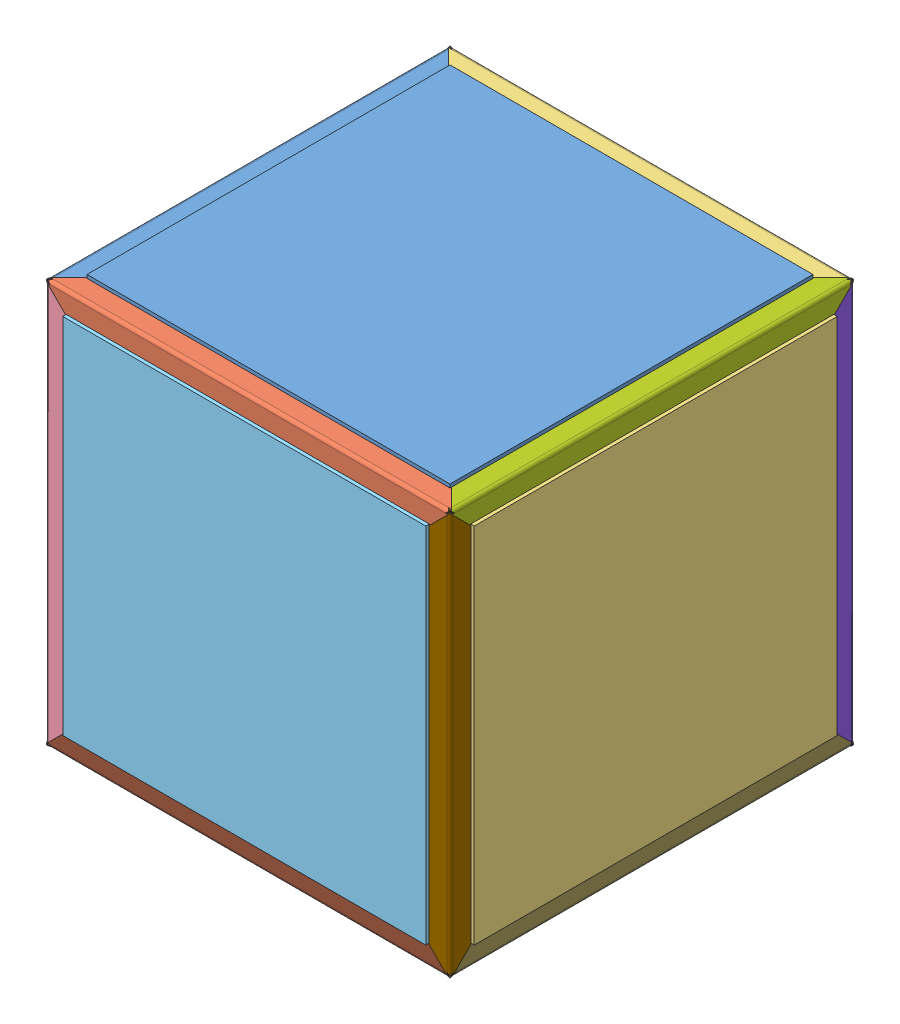
SolidWorks assembly cube_36, configuration cube36. Lengths in mm.
Overall size (188.59 188.59 188.59).
30 component instances, 30 part files, 93 mates.
Components (placement in the parent):
- pr^cube_36-28: pr^cube_36 [cube01] x (-1 0 0) z (0 0 1) size (166.37 1.59 166.37) (virtual)
- pg^cube_36-20: pg^cube_36 [cube01] x (0 -1 0) z (0 0 1) size (166.37 1.59 166.37) (virtual)
- po^cube_36-22: po^cube_36 [cube01] x (0 1 0) z (0 0 1) size (166.37 1.59 166.37) (virtual)
- py^cube_36-21: py^cube_36 [cube01] at origin size (166.37 1.59 166.37) (virtual)
- pc^cube_36-18: pc^cube_36 [cube01] x (-1 0 0) z (0 -1 0) size (166.37 1.59 166.37) (virtual)
- pb^cube_36-21: pb^cube_36 [cube01] x (-1 0 0) z (0 1 0) size (166.37 1.59 166.37) (virtual)
- br1^cube_36-49: br1^cube_36 [Default] at (0 67.31 -67.31) x (0 0 1) z (-1 0 0) size (50.8 50.8 127.51) (virtual)
- br2^cube_36-61: br2^cube_36 [Default] at (-67.31 67.31 0) size (50.8 50.8 127.51) (virtual)
- br3^cube_36-46: br3^cube_36 [Default] at (0 67.31 67.31) x (0 0 -1) z (1 0 0) size (50.8 50.8 127.51) (virtual)
- bg1^cube_36-47: bg1^cube_36 [Default] at (-67.31 -67.31 0) x (0 1 0) z (0 0 1) size (50.8 50.8 127.51) (virtual)
- bg2^cube_36-44: bg2^cube_36 [Default] at (-67.31 0 67.31) x (0 0 -1) z (0 1 0) size (50.8 50.8 127.51) (virtual)
- bg3^cube_36-40: bg3^cube_36 [Default] at (-67.31 0 -67.31) x (0 0 1) z (0 -1 0) size (50.8 50.8 127.51) (virtual)
- bo1^cube_36-42: bo1^cube_36 [Default] at (67.31 0 -67.31) x (0 0 1) z (0 1 0) size (50.8 50.8 127.51) (virtual)
- bo2^cube_36-46: bo2^cube_36 [Default] at (67.31 0 67.31) x (0 0 -1) z (0 -1 0) size (50.8 50.8 127.51) (virtual)
- bo3^cube_36-62: bo3^cube_36 [Default] at (67.31 67.31 0) x (0 -1 0) z (0 0 1) size (50.8 50.8 127.51) (virtual)
- by1^cube_36-41: by1^cube_36 [Default] at (0 -67.31 -67.31) x (0 0 1) z (1 0 0) size (50.8 50.8 127.51) (virtual)
- by2^cube_36-45: by2^cube_36 [Default] at (0 -67.31 67.31) x (0 0 -1) z (-1 0 0) size (50.8 50.8 127.51) (virtual)
- by3^cube_36-48: by3^cube_36 [Default] at (67.31 -67.31 0) x (-1 0 0) z (0 0 1) size (50.8 50.8 127.51) (virtual)
- dr1^cube_36-55: dr1^cube_36 [cube01] at (-92.1046 92.71 0) x (0 -1 0) z (0 0 1) size (26.01 26.01 185.43) (hidden, virtual)
- dr2^cube_36-37: dr2^cube_36 [cube01] at (0 92.71 92.1046) x (0 -1 0) z (1 0 0) size (26.01 26.01 185.43) (hidden, virtual)
- dr3^cube_36-33: dr3^cube_36 [cube01] at (0 92.71 -92.1046) x (0 -1 0) z (-1 0 0) size (26.01 26.01 185.43) (hidden, virtual)
- dg1^cube_36-38: dg1^cube_36 [cube01] at (-92.71 0 92.1046) x (1 0 0) z (0 1 0) size (26.01 26.01 185.43) (hidden, virtual)
- dg2^cube_36-41: dg2^cube_36 [cube01] at (-92.71 -92.1046 0) size (26.01 26.01 185.43) (hidden, virtual)
- dg3^cube_36-34: dg3^cube_36 [cube01] at (-92.71 0 -92.1046) x (1 0 0) z (0 -1 0) size (26.01 26.01 185.43) (hidden, virtual)
- do3^cube_36-47: do3^cube_36 [cube01] at (92.71 92.1046 0) x (-1 0 0) z (0 0 1) size (26.01 26.01 185.43) (hidden, virtual)
- do1^cube_36-36: do1^cube_36 [cube01] at (92.71 0 -92.1046) x (-1 0 0) z (0 1 0) size (26.01 26.01 185.43) (hidden, virtual)
- do2^cube_36-40: do2^cube_36 [cube01] at (92.71 0 92.1046) x (-1 0 0) z (0 -1 0) size (26.01 26.01 185.43) (hidden, virtual)
- dy1^cube_36-35: dy1^cube_36 [cube01] at (0 -92.71 -92.1046) x (0 1 0) z (1 0 0) size (26.01 26.01 185.43) (hidden, virtual)
- dy2^cube_36-39: dy2^cube_36 [cube01] at (0 -92.71 92.1046) x (0 1 0) z (-1 0 0) size (26.01 26.01 185.43) (hidden, virtual)
- dy3^cube_36-42: dy3^cube_36 [cube01] at (92.1046 -92.71 0) x (0 1 0) z (0 0 1) size (26.01 26.01 185.43) (hidden, virtual)
Mates (geometry in assembly coordinates):
- Coincident1: coincident anti-aligned: plane of pr^cube_36-28 through (83.185 92.71 -83.185) normal (0 -1 0); plane of br1^cube_36-49 through (-63.754 92.71 -67.31) normal (0 1 0)
- Coincident2: coincident anti-aligned: plane of pr^cube_36-28 through (83.185 92.71 -83.185) normal (0 -1 0); plane of br2^cube_36-61 through (-67.31 92.71 63.754) normal (0 1 0)
- Coincident3: coincident anti-aligned: plane of pr^cube_36-28 through (83.185 92.71 -83.185) normal (0 -1 0); plane of br3^cube_36-46 through (63.754 92.71 67.31) normal (0 1 0)
- Coincident4: coincident anti-aligned: plane of pr^cube_36-28 through (83.185 92.71 -83.185) normal (0 -1 0); plane of bo3^cube_36-62 through (67.31 92.71 63.754) normal (0 1 0)
- Coincident5: coincident anti-aligned: plane of pr^cube_36-28 through (83.185 92.71 -83.185) normal (0 -1 0); plane of dr3^cube_36-33 through (0 92.71 -184.8146) normal (0 1 0)
- Coincident6: coincident anti-aligned: plane of pr^cube_36-28 through (83.185 92.71 -83.185) normal (0 -1 0); plane of dr1^cube_36-55 through (-184.8146 92.71 0) normal (0 1 0)
- Coincident7: coincident anti-aligned: plane of pr^cube_36-28 through (83.185 92.71 -83.185) normal (0 -1 0); plane of do3^cube_36-47 through (-0.6054 92.71 0) normal (0 1 0)
- Coincident8: coincident anti-aligned: plane of pr^cube_36-28 through (83.185 92.71 -83.185) normal (0 -1 0); plane of dr2^cube_36-37 through (0 92.71 184.8146) normal (0 1 0)
- Coincident34: coincident anti-aligned: plane of pb^cube_36-21 through (83.185 -83.185 -92.71) normal (0 0 1); plane of by1^cube_36-41 through (63.754 -67.31 -92.71) normal (0 0 -1)
- Coincident35: coincident anti-aligned: plane of pb^cube_36-21 through (83.185 -83.185 -92.71) normal (0 0 1); plane of bo1^cube_36-42 through (67.31 63.754 -92.71) normal (0 0 -1)
- Coincident36: coincident anti-aligned: plane of pb^cube_36-21 through (83.185 -83.185 -92.71) normal (0 0 1); plane of br1^cube_36-49 through (-63.754 67.31 -92.71) normal (0 0 -1)
- Coincident37: coincident anti-aligned: plane of pb^cube_36-21 through (83.185 -83.185 -92.71) normal (0 0 1); plane of bg3^cube_36-40 through (-67.31 -63.754 -92.71) normal (0 0 -1)
- Coincident38: coincident anti-aligned: plane of pb^cube_36-21 through (83.185 -83.185 -92.71) normal (0 0 1); plane of dg3^cube_36-34 through (0.6054 0 -92.71) normal (0 0 -1)
- Coincident39: coincident anti-aligned: plane of pb^cube_36-21 through (83.185 -83.185 -92.71) normal (0 0 1); plane of dr3^cube_36-33 through (0 -0.6054 -92.71) normal (0 0 -1)
- Coincident40: coincident anti-aligned: plane of pb^cube_36-21 through (83.185 -83.185 -92.71) normal (0 0 1); plane of do1^cube_36-36 through (-0.6054 0 -92.71) normal (0 0 -1)
- Coincident41: coincident anti-aligned: plane of pb^cube_36-21 through (83.185 -83.185 -92.71) normal (0 0 1); plane of dy1^cube_36-35 through (0 0.6054 -92.71) normal (0 0 -1)
- Coincident42: coincident anti-aligned: plane of pc^cube_36-18 through (83.185 83.185 92.71) normal (0 0 -1); plane of bo2^cube_36-46 through (67.31 -63.754 92.71) normal (0 0 1)
- Coincident43: coincident anti-aligned: plane of pc^cube_36-18 through (83.185 83.185 92.71) normal (0 0 -1); plane of br3^cube_36-46 through (63.754 67.31 92.71) normal (0 0 1)
- Coincident44: coincident anti-aligned: plane of pc^cube_36-18 through (83.185 83.185 92.71) normal (0 0 -1); plane of bg2^cube_36-44 through (-67.31 63.754 92.71) normal (0 0 1)
- Coincident45: coincident anti-aligned: plane of pc^cube_36-18 through (83.185 83.185 92.71) normal (0 0 -1); plane of by2^cube_36-45 through (-63.754 -67.31 92.71) normal (0 0 1)
- Coincident46: coincident anti-aligned: plane of pc^cube_36-18 through (83.185 83.185 92.71) normal (0 0 -1); plane of do2^cube_36-40 through (-0.6054 0 92.71) normal (0 0 1)
- Coincident47: coincident anti-aligned: plane of pc^cube_36-18 through (83.185 83.185 92.71) normal (0 0 -1); plane of dy2^cube_36-39 through (0 0.6054 92.71) normal (0 0 1)
- Coincident48: coincident anti-aligned: plane of pc^cube_36-18 through (83.185 83.185 92.71) normal (0 0 -1); plane of dg1^cube_36-38 through (0.6054 0 92.71) normal (0 0 1)
- Coincident49: coincident anti-aligned: plane of pc^cube_36-18 through (83.185 83.185 92.71) normal (0 0 -1); plane of dr2^cube_36-37 through (0 -0.6054 92.71) normal (0 0 1)
- Coincident50: coincident anti-aligned: plane of pg^cube_36-20 through (-92.71 83.185 -83.185) normal (1 0 0); plane of bg3^cube_36-40 through (-92.71 -63.754 -67.31) normal (-1 0 0)
- Coincident51: coincident anti-aligned: plane of pg^cube_36-20 through (-92.71 83.185 -83.185) normal (1 0 0); plane of bg1^cube_36-47 through (-92.71 -67.31 63.754) normal (-1 0 0)
- Coincident52: coincident anti-aligned: plane of pg^cube_36-20 through (-92.71 83.185 -83.185) normal (1 0 0); plane of bg2^cube_36-44 through (-92.71 63.754 67.31) normal (-1 0 0)
- Coincident53: coincident anti-aligned: plane of pg^cube_36-20 through (-92.71 83.185 -83.185) normal (1 0 0); plane of dr1^cube_36-55 through (-92.71 -0.6054 0) normal (-1 0 0)
- Coincident54: coincident anti-aligned: plane of pg^cube_36-20 through (-92.71 83.185 -83.185) normal (1 0 0); plane of dg3^cube_36-34 through (-92.71 0 -184.8146) normal (-1 0 0)
- Coincident55: coincident anti-aligned: plane of pg^cube_36-20 through (-92.71 83.185 -83.185) normal (1 0 0); plane of dg2^cube_36-41 through (-92.71 -184.8146 0) normal (-1 0 0)
- Coincident56: coincident anti-aligned: plane of pg^cube_36-20 through (-92.71 83.185 -83.185) normal (1 0 0); plane of dg1^cube_36-38 through (-92.71 0 184.8146) normal (-1 0 0)
- Coincident99: coincident anti-aligned: plane of pg^cube_36-20 through (-92.71 83.185 -83.185) normal (1 0 0); plane of br2^cube_36-61 through (-92.71 67.31 63.754) normal (-1 0 0)
- Coincident57: coincident anti-aligned: plane of py^cube_36-21 through (-83.185 -92.71 -83.185) normal (0 1 0); plane of by3^cube_36-48 through (67.31 -92.71 63.754) normal (0 -1 0)
- Coincident58: coincident anti-aligned: plane of py^cube_36-21 through (-83.185 -92.71 -83.185) normal (0 1 0); plane of by2^cube_36-45 through (-63.754 -92.71 67.31) normal (0 -1 0)
- Coincident59: coincident anti-aligned: plane of py^cube_36-21 through (-83.185 -92.71 -83.185) normal (0 1 0); plane of bg1^cube_36-47 through (-67.31 -92.71 63.754) normal (0 -1 0)
- Coincident60: coincident anti-aligned: plane of py^cube_36-21 through (-83.185 -92.71 -83.185) normal (0 1 0); plane of by1^cube_36-41 through (63.754 -92.71 -67.31) normal (0 -1 0)
- Coincident61: coincident anti-aligned: plane of py^cube_36-21 through (-83.185 -92.71 -83.185) normal (0 1 0); plane of dy3^cube_36-42 through (184.8146 -92.71 0) normal (0 -1 0)
- Coincident62: coincident anti-aligned: plane of py^cube_36-21 through (-83.185 -92.71 -83.185) normal (0 1 0); plane of dy2^cube_36-39 through (0 -92.71 184.8146) normal (0 -1 0)
- Coincident63: coincident anti-aligned: plane of py^cube_36-21 through (-83.185 -92.71 -83.185) normal (0 1 0); plane of dg2^cube_36-41 through (0.6054 -92.71 0) normal (0 -1 0)
- Coincident64: coincident anti-aligned: plane of py^cube_36-21 through (-83.185 -92.71 -83.185) normal (0 1 0); plane of dy1^cube_36-35 through (0 -92.71 -184.8146) normal (0 -1 0)
- Coincident65: coincident anti-aligned: plane of po^cube_36-22 through (92.71 -83.185 -83.185) normal (-1 0 0); plane of bo1^cube_36-42 through (92.71 63.754 -67.31) normal (1 0 0)
- Coincident66: coincident anti-aligned: plane of po^cube_36-22 through (92.71 -83.185 -83.185) normal (-1 0 0); plane of by3^cube_36-48 through (92.71 -67.31 63.754) normal (1 0 0)
- Coincident67: coincident anti-aligned: plane of po^cube_36-22 through (92.71 -83.185 -83.185) normal (-1 0 0); plane of bo2^cube_36-46 through (92.71 -63.754 67.31) normal (1 0 0)
- Coincident68: coincident anti-aligned: plane of po^cube_36-22 through (92.71 -83.185 -83.185) normal (-1 0 0); plane of bo3^cube_36-62 through (92.71 67.31 63.754) normal (1 0 0)
- Coincident69: coincident anti-aligned: plane of po^cube_36-22 through (92.71 -83.185 -83.185) normal (-1 0 0); plane of do2^cube_36-40 through (92.71 0 184.8146) normal (1 0 0)
- Coincident70: coincident anti-aligned: plane of po^cube_36-22 through (92.71 -83.185 -83.185) normal (-1 0 0); plane of do3^cube_36-47 through (92.71 184.8146 0) normal (1 0 0)
- Coincident71: coincident anti-aligned: plane of po^cube_36-22 through (92.71 -83.185 -83.185) normal (-1 0 0); plane of do1^cube_36-36 through (92.71 0 -184.8146) normal (1 0 0)
- Coincident72: coincident anti-aligned: plane of po^cube_36-22 through (92.71 -83.185 -83.185) normal (-1 0 0); plane of dy3^cube_36-42 through (92.71 0.6054 0) normal (1 0 0)
- Coincident73: coincident aligned: plane of assembly through (0 0 0) normal (0 0 1); plane of dy3^cube_36-42 through (92.1046 -92.71 0) normal (0 0 1)
- Coincident74: coincident aligned: plane of assembly through (0 0 0) normal (0 0 1); plane of by3^cube_36-48 through (67.31 -67.31 0) normal (0 0 1)
- Coincident75: coincident aligned: plane of assembly through (0 0 0) normal (0 0 1); plane of bo3^cube_36-62 through (67.31 67.31 0) normal (0 0 1)
- Coincident76: coincident aligned: plane of assembly through (0 0 0) normal (0 0 1); plane of do3^cube_36-47 through (92.71 92.1046 0) normal (0 0 1)
- Coincident77: coincident aligned: plane of assembly through (0 0 0) normal (0 0 1); plane of dg2^cube_36-41 through (-92.71 -92.1046 0) normal (0 0 1)
- Coincident78: coincident aligned: plane of assembly through (0 0 0) normal (0 0 1); plane of bg1^cube_36-47 through (-67.31 -67.31 0) normal (0 0 1)
- Coincident79: coincident aligned: plane of assembly through (0 0 0) normal (0 0 1); plane of dr1^cube_36-55 through (-92.1046 92.71 0) normal (0 0 1)
- Coincident80: coincident aligned: plane of assembly through (0 0 0) normal (0 0 1); plane of br2^cube_36-61 through (-67.31 67.31 0) normal (0 0 1)
- Coincident81: coincident aligned: plane of assembly through (0 0 0) normal (0 1 0); plane of bo1^cube_36-42 through (67.31 0 -67.31) normal (0 1 0)
- Coincident82: coincident aligned: plane of assembly through (0 0 0) normal (0 1 0); plane of py^cube_36-21 through (0 0 0) normal (0 1 0)
- Coincident83: coincident aligned: plane of assembly through (0 0 0) normal (0 1 0); plane of do1^cube_36-36 through (92.71 0 -92.1046) normal (0 1 0)
- Coincident84: coincident anti-aligned: plane of assembly through (0 0 0) normal (0 1 0); plane of bg3^cube_36-40 through (-67.31 0 -67.31) normal (0 -1 0)
- Coincident85: coincident anti-aligned: plane of assembly through (0 0 0) normal (0 1 0); plane of dg3^cube_36-34 through (-92.71 0 -92.1046) normal (0 -1 0)
- Coincident86: coincident aligned: plane of assembly through (0 0 0) normal (0 1 0); plane of dg1^cube_36-38 through (-92.71 0 92.1046) normal (0 1 0)
- Coincident87: coincident aligned: plane of assembly through (0 0 0) normal (0 1 0); plane of bg2^cube_36-44 through (-67.31 0 67.31) normal (0 1 0)
- Coincident88: coincident anti-aligned: plane of assembly through (0 0 0) normal (0 1 0); plane of bo2^cube_36-46 through (67.31 0 67.31) normal (0 -1 0)
- Coincident89: coincident anti-aligned: plane of assembly through (0 0 0) normal (0 1 0); plane of do2^cube_36-40 through (92.71 0 92.1046) normal (0 -1 0)
- Coincident90: coincident anti-aligned: plane of assembly through (0 0 0) normal (1 0 0); plane of by2^cube_36-45 through (0 -67.31 67.31) normal (-1 0 0)
- Coincident91: coincident anti-aligned: plane of assembly through (0 0 0) normal (1 0 0); plane of dy2^cube_36-39 through (0 -92.71 92.1046) normal (-1 0 0)
- Coincident92: coincident aligned: plane of assembly through (0 0 0) normal (1 0 0); plane of pg^cube_36-20
- Coincident93: coincident aligned: plane of assembly through (0 0 0) normal (1 0 0); plane of dr2^cube_36-37 through (0 92.71 92.1046) normal (1 0 0)
- Coincident94: coincident aligned: plane of assembly through (0 0 0) normal (1 0 0); plane of br3^cube_36-46 through (0 67.31 67.31) normal (1 0 0)
- Coincident95: coincident anti-aligned: plane of assembly through (0 0 0) normal (1 0 0); plane of dr3^cube_36-33 through (0 92.71 -92.1046) normal (-1 0 0)
- Coincident96: coincident anti-aligned: plane of assembly through (0 0 0) normal (1 0 0); plane of br1^cube_36-49 through (0 67.31 -67.31) normal (-1 0 0)
- Coincident97: coincident aligned: plane of assembly through (0 0 0) normal (1 0 0); plane of by1^cube_36-41 through (0 -67.31 -67.31) normal (1 0 0)
- Coincident98: coincident aligned: plane of assembly through (0 0 0) normal (1 0 0); plane of dy1^cube_36-35 through (0 -92.71 -92.1046) normal (1 0 0)
- Coincident100: coincident anti-aligned: plane of pr^cube_36-28; plane of assembly through (0 0 0) normal (1 0 0)
- Coincident101: coincident aligned: plane of pr^cube_36-28 through (0 0 0) normal (0 0 1); plane of assembly through (0 0 0) normal (0 0 1)
- Coincident102: coincident anti-aligned: plane of pr^cube_36-28; plane of assembly through (0 0 0) normal (0 1 0)
- Coincident106: coincident anti-aligned: plane of pg^cube_36-20; plane of assembly through (0 0 0) normal (0 1 0)
- Coincident107: coincident aligned: plane of pg^cube_36-20; plane of assembly through (0 0 0) normal (1 0 0)
- Coincident108: coincident aligned: plane of pg^cube_36-20 through (0 0 0) normal (0 0 1); plane of assembly through (0 0 0) normal (0 0 1)
- Coincident109: coincident aligned: plane of py^cube_36-21 through (0 0 0) normal (0 0 1); plane of assembly through (0 0 0) normal (0 0 1)
- Coincident110: coincident aligned: plane of py^cube_36-21 through (0 0 0) normal (0 1 0); plane of assembly through (0 0 0) normal (0 1 0)
- Coincident111: coincident aligned: plane of py^cube_36-21 through (0 0 0) normal (1 0 0); plane of assembly through (0 0 0) normal (1 0 0)
- Coincident112: coincident aligned: plane of po^cube_36-22 through (0 0 0) normal (0 0 1); plane of assembly through (0 0 0) normal (0 0 1)
- Coincident113: coincident anti-aligned: plane of po^cube_36-22; plane of assembly through (0 0 0) normal (1 0 0)
- Coincident114: coincident aligned: plane of po^cube_36-22; plane of assembly through (0 0 0) normal (0 1 0)
- Coincident115: coincident anti-aligned: plane of pc^cube_36-18 through (0 0 0) normal (0 -1 0); plane of assembly through (0 0 0) normal (0 1 0)
- Coincident116: coincident anti-aligned: plane of pc^cube_36-18; plane of assembly through (0 0 0) normal (0 0 1)
- Coincident117: coincident anti-aligned: plane of pc^cube_36-18; plane of assembly through (0 0 0) normal (1 0 0)
- Coincident118: coincident aligned: plane of pb^cube_36-21 through (0 0 0) normal (0 1 0); plane of assembly through (0 0 0) normal (0 1 0)
- Coincident119: coincident aligned: plane of pb^cube_36-21; plane of assembly through (0 0 0) normal (0 0 1)
- Coincident120: coincident anti-aligned: line of pb^cube_36-21 through (0.8731 -0.8731 0) axis (0 0 -1); sketch_entity of pr^cube_36-28; plane of pb^cube_36-21 through (83.185 -83.185 -94.2975) normal (0 0 -1); plane of py^cube_36-21 through (-83.185 -94.2975 -83.185) normal (0 -1 0)
- cyan_cut: unknown: unknown of pc^cube_36-18; plane of pc^cube_36-18 through (83.185 83.185 94.2975) normal (0 0 1); plane of pg^cube_36-20 through (-94.2975 83.185 -83.185) normal (-1 0 0); plane of po^cube_36-22 through (94.2975 -83.185 -83.185) normal (1 0 0)
